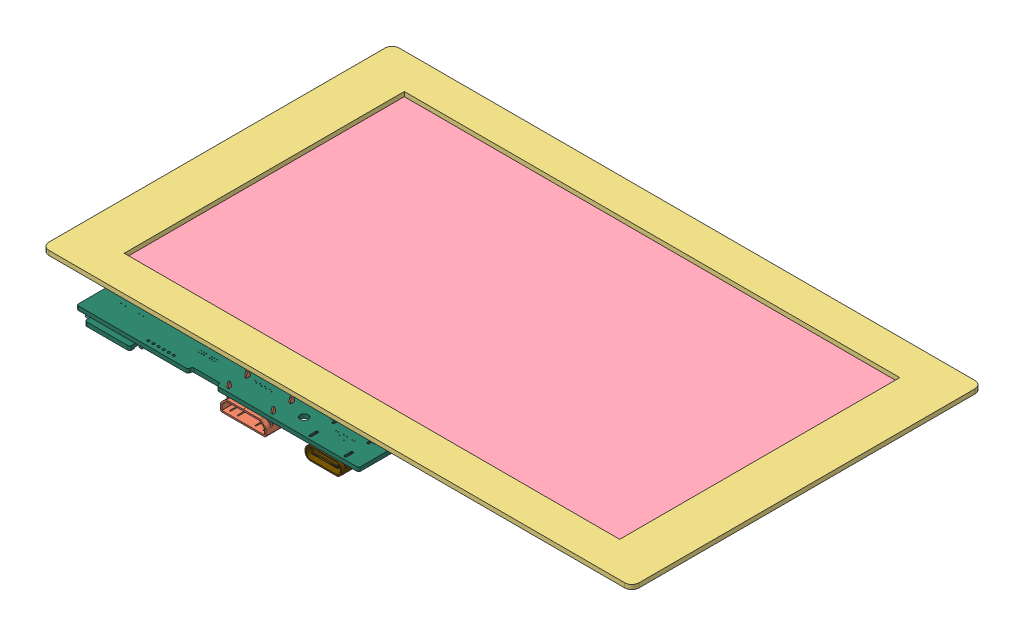
SolidWorks assembly Assembly Center Components, configuration Default. Lengths in mm.
Overall size (146.77 13.35 93.89).
640 component instances, 141 part files, 3 mates.
Components (placement in the parent):
- Mini HDMI 685119136923-1: Mini HDMI 685119136923 [Default] at (-19.19 -7.55 40.38) x (0 0 1) z (0 -1 0) size (7.9 11.25 5.45)
  - Mini HDMI 685119136923(1)-1: Mini HDMI 685119136923(1) [Default] at origin size (7.9 11.25 5.45)
    - Housing-1: Housing [Default] at origin size (5.5 11.25 2.9)
    - Shielding-1: Shielding [Default] at (2.875 0 0.82) x (0 1 0) z (0 0 1) size (11.21 7.6 5.45)
    - Housing2-1: Housing2 [Default] at (-0.075 0 -0.65) x (0 -1 0) z (0 0 1) size (8.25 0.75 1.6)
    - Pin1-1: Pin1 [Default] at (2.1 -3.6 0.3) size (5.9 0.15 1.8)
    - Pin1-2: Pin1 [Default] at (2.1 -2.8 0.3) size (5.9 0.15 1.8)
    - Pin1-3: Pin1 [Default] at (2.1 -2.4 0.3) size (5.9 0.15 1.8)
    - Pin1-4: Pin1 [Default] at (2.1 -2 0.3) size (5.9 0.15 1.8)
    - Pin1-5: Pin1 [Default] at (2.1 -1.6 0.3) size (5.9 0.15 1.8)
    - Pin1-6: Pin1 [Default] at (2.1 -1.2 0.3) size (5.9 0.15 1.8)
    - Pin1-7: Pin1 [Default] at (2.1 -0.8 0.3) size (5.9 0.15 1.8)
    - Pin1-8: Pin1 [Default] at (2.1 -0.4 0.3) size (5.9 0.15 1.8)
    - Pin1-9: Pin1 [Default] at (2.1 0 0.3) size (5.9 0.15 1.8)
    - Pin1-10: Pin1 [Default] at (2.1 0.4 0.3) size (5.9 0.15 1.8)
    - Pin1-11: Pin1 [Default] at (2.1 0.8 0.3) size (5.9 0.15 1.8)
    - Pin1-12: Pin1 [Default] at (2.1 1.2 0.3) size (5.9 0.15 1.8)
    - Pin1-13: Pin1 [Default] at (2.1 1.6 0.3) size (5.9 0.15 1.8)
    - Pin1-14: Pin1 [Default] at (2.1 2 0.3) size (5.9 0.15 1.8)
    - Pin1-15: Pin1 [Default] at (2.1 2.4 0.3) size (5.9 0.15 1.8)
    - Pin1-16: Pin1 [Default] at (2.1 2.8 0.3) size (5.9 0.15 1.8)
    - Pin1-17: Pin1 [Default] at (2.1 3.2 0.3) size (5.9 0.15 1.8)
    - Pin1-18: Pin1 [Default] at (2.1 3.6 0.3) size (5.9 0.15 1.8)
    - Pin2-1: Pin2 [Default] at (1.7983 -3.2 0.3) size (5.3 0.15 1.8)
- AX210 PCIe Card-1: AX210 PCIe Card [Default] at (0 25.3 -0.4) size (22 0.1 30)
  - Component473-1: Component473 [Default] at origin size (0.15 0.02 2.3)
  - Component424-1: Component424 [Default] at origin size (0.15 0.02 2.3)
  - Component429-1: Component429 [Default] at origin size (0.15 0.02 2.3)
  - Component423-1: Component423 [Default] at origin size (0.15 0.02 2.3)
  - Component430-1: Component430 [Default] at origin size (0.15 0.02 2.3)
  - Component431-1: Component431 [Default] at origin size (0.15 0.02 2.3)
  - Component426-1: Component426 [Default] at origin size (0.15 0.02 2.3)
  - Component422-1: Component422 [Default] at origin size (0.15 0.02 2.3)
  - Component425-1: Component425 [Default] at origin size (0.15 0.02 2.3)
  - Component428-1: Component428 [Default] at origin size (0.15 0.02 2.3)
  - Component446-1: Component446 [Default] at origin size (0.15 0.02 2.3)
  - Component448-1: Component448 [Default] at origin size (0.15 0.02 2.3)
  - Component449-1: Component449 [Default] at origin size (0.15 0.02 2.3)
  - Component443-1: Component443 [Default] at origin size (0.15 0.02 2.3)
  - Component442-1: Component442 [Default] at origin size (0.15 0.02 2.3)
  - Component447-1: Component447 [Default] at origin size (0.15 0.02 2.3)
  - Component451-1: Component451 [Default] at origin size (0.15 0.02 2.3)
  - Component450-1: Component450 [Default] at origin size (0.15 0.02 2.3)
  - Component445-1: Component445 [Default] at origin size (0.15 0.02 2.3)
  - Component472-1: Component472 [Default] at origin size (0.15 0.02 2.3)
  - Component408-1: Component408 [Default] at origin size (0.15 0.02 2.3)
  - Component409-1: Component409 [Default] at origin size (0.15 0.02 2.3)
  - Component410-1: Component410 [Default] at origin size (0.15 0.02 2.3)
  - Component405-1: Component405 [Default] at origin size (0.15 0.02 2.3)
  - Component411-1: Component411 [Default] at origin size (0.15 0.02 2.3)
  - Component403-1: Component403 [Default] at origin size (0.15 0.02 2.3)
  - Component406-1: Component406 [Default] at origin size (0.15 0.02 2.3)
  - Component404-1: Component404 [Default] at origin size (0.15 0.02 2.3)
  - Component407-1: Component407 [Default] at origin size (0.15 0.02 2.3)
  - Component400-1: Component400 [Default] at origin size (0.15 0.02 2.3)
  - Component401-1: Component401 [Default] at origin size (0.15 0.02 2.3)
  - Component433-1: Component433 [Default] at origin size (0.15 0.02 2.3)
  - Component437-1: Component437 [Default] at origin size (0.15 0.02 2.3)
  - Component438-1: Component438 [Default] at origin size (0.15 0.02 2.3)
  - Component436-1: Component436 [Default] at origin size (0.15 0.02 2.3)
  - Component434-1: Component434 [Default] at origin size (0.15 0.02 2.3)
  - Component439-1: Component439 [Default] at origin size (0.15 0.02 2.3)
  - Component440-1: Component440 [Default] at origin size (0.15 0.02 2.3)
  - Component435-1: Component435 [Default] at origin size (0.15 0.02 2.3)
  - Component458-1: Component458 [Default] at origin size (0.15 0.02 2.3)
  - Component460-1: Component460 [Default] at origin size (0.15 0.02 2.3)
  - Component456-1: Component456 [Default] at origin size (0.15 0.02 2.3)
  - Component457-1: Component457 [Default] at origin size (0.15 0.02 2.3)
  - Component461-1: Component461 [Default] at origin size (0.15 0.02 2.3)
  - Component452-1: Component452 [Default] at origin size (0.15 0.02 2.3)
  - Component453-1: Component453 [Default] at origin size (0.15 0.02 2.3)
  - Component455-1: Component455 [Default] at origin size (0.15 0.02 2.3)
  - Component465-1: Component465 [Default] at origin size (0.15 0.02 2.3)
  - Component468-1: Component468 [Default] at origin size (0.15 0.02 2.3)
  - Component467-1: Component467 [Default] at origin size (0.15 0.02 2.3)
  - Component464-1: Component464 [Default] at origin size (0.15 0.02 2.3)
  - Component469-1: Component469 [Default] at origin size (0.15 0.02 2.3)
  - Component470-1: Component470 [Default] at origin size (0.15 0.02 2.3)
  - Component471-1: Component471 [Default] at origin size (0.15 0.02 2.3)
  - Component462-1: Component462 [Default] at origin size (0.15 0.02 2.3)
  - Component463-1: Component463 [Default] at origin size (0.15 0.02 2.3)
  - Component466-1: Component466 [Default] at origin size (0.15 0.02 2.3)
  - Component413-1: Component413 [Default] at origin size (0.15 0.02 2.3)
  - Component417-1: Component417 [Default] at origin size (0.15 0.02 2.3)
  - Component414-1: Component414 [Default] at origin size (0.15 0.02 2.3)
  - Component415-1: Component415 [Default] at origin size (0.15 0.02 2.3)
  - Component421-1: Component421 [Default] at origin size (0.15 0.02 2.3)
  - Component418-1: Component418 [Default] at origin size (0.15 0.02 2.3)
  - Component419-1: Component419 [Default] at origin size (0.15 0.02 2.3)
  - Component420-1: Component420 [Default] at origin size (0.15 0.02 2.3)
  - Component412-1: Component412 [Default] at origin size (0.15 0.02 2.3)
  - AX210 PCIe Card-0-1: AX210 PCIe Card-0 [Default] at origin size (0.15 0.02 2.3)
  - AX210 PCIe Card-1-1: AX210 PCIe Card-1 [Default] at origin size (5.53 0.08 2.73)
  - AX210 PCIe Card-2-1: AX210 PCIe Card-2 [Default] at origin size (22 0.08 30)
- 5.5_ Touch Display MIPI-1: 5.5_ Touch Display MIPI [Default] at origin size (145.01 5.25 86.09)
  - CTP-1: CTP [Default] at origin size (145.01 1.1 86.09)
  - 5.5_ Touch Display MIPI-3-1: 5.5_ Touch Display MIPI-3 [Default] at origin size (133.31 3.65 74.36)
  - 5.5_ Touch Display MIPI-4-1: 5.5_ Touch Display MIPI-4 [Default] at origin size (45 0.5 15.5)
  - 5.5_ Touch Display MIPI-5-1: 5.5_ Touch Display MIPI-5 [Default] at origin size (53.5 0.5 4.5)
- RNQ0040A v1-1: RNQ0040A v1 [Default] at (1.8323 -6.1 22.7032) x (1 0 0) z (0 -1 0) size (6 4 0.8)
  - BODY-QFN-1: BODY-QFN [Default] at (0 0 0.025) x (1 0 0) z (0 -1 0) size (6 0.78 4)
  - FRAME-RNQ0040A-1: FRAME-RNQ0040A [Default] x (1 0 0) z (0 -1 0) size (6 0.2 4)
- Radxa CM3-1: Radxa CM3 [Default] at (-34.1679 -8.7691 -17.6603) x (0 0 -1) z (0 -1 0) size (40.05 55.02 3.7)
  - Board_Geoms-1: Board_Geoms [Default] at origin size (40.05 55.02 1.2)
    - Board_outline-1: Board_outline [Default] at origin size (40.05 55.02 1.2)
  - EMP_Models-1: EMP_Models [Default] at origin size (39.5 54.73 3.7)
    - ANT2-1: ANT2 [Default] at (-11.75 25.8 0) size (4.01 3.43 1.3)
    - C1-1: C1 [Default] at (-3.8475 -1.7481 -1.2) x (-0.707107 -0.707107 0) z (0 0 -1) size (1.7 0.9 0.5)
    - C10-1: C10 [Default] at (3.3025 0.0519 -1.2) x (0.707107 0.707107 0) z (0 0 -1) size (1.1 0.6 0.35)
    - C10-2: C10 [Default] at (10.95 15.45 -1.2) x (0 1 0) z (0 0 -1) size (1.1 0.6 0.35)
    - C10-3: C10 [Default] at (3.8025 -0.3981 -1.2) x (-0.707107 -0.707107 0) z (0 0 -1) size (1.1 0.6 0.35)
    - C10-4: C10 [Default] at (-3.9975 -0.8481 -1.2) x (0.707107 0.707107 0) z (0 0 -1) size (1.1 0.6 0.35)
    - C1-2: C1 [Default] at (-14.1389 2.0823 0) x (0 1 0) z (0 0 1) size (1.7 0.9 0.5)
    - C10-5: C10 [Default] at (-4.6975 -21.9981 -1.2) x (0.707107 0.707107 0) z (0 0 -1) size (1.1 0.6 0.35)
    - C105-1: C105 [Default] at (13.9593 20.2111 -1.2) x (1 0 0) z (0 0 -1) size (2.5 1.3 0.6)
    - C105-2: C105 [Default] at (0.7006 -26.6671 0) size (2.5 1.3 0.6)
    - C105-3: C105 [Default] at (3.9693 -10.6117 -1.2) x (0 1 0) z (0 0 -1) size (2.5 1.3 0.6)
    - C10-6: C10 [Default] at (-3.0975 -8.9981 -1.2) x (0 1 0) z (0 0 -1) size (1.1 0.6 0.35)
    - C10-7: C10 [Default] at (-2.3475 -3.2981 -1.2) x (-0.707107 -0.707107 0) z (0 0 -1) size (1.1 0.6 0.35)
    - C1-3: C1 [Default] at (3.0025 0.7019 -1.2) x (0.707107 0.707107 0) z (0 0 -1) size (1.7 0.9 0.5)
    - C10-8: C10 [Default] at (-1.4475 -4.5481 -1.2) x (-0.707107 -0.707107 0) z (0 0 -1) size (1.1 0.6 0.35)
    - C10-9: C10 [Default] at (0.4525 -5.1481 -1.2) x (-0.707107 -0.707107 0) z (0 0 -1) size (1.1 0.6 0.35)
    - C10-10: C10 [Default] at (1.1525 -20.3481 -1.2) x (0 1 0) z (0 0 -1) size (1.1 0.6 0.35)
    - C10-11: C10 [Default] at (-2.0975 -16.8481 -1.2) x (0 1 0) z (0 0 -1) size (1.1 0.6 0.35)
    - C10-12: C10 [Default] at (-8.6975 -22.5481 -1.2) x (0.707107 -0.707107 0) z (0 0 -1) size (1.1 0.6 0.35)
    - C10-13: C10 [Default] at (-1.7475 -19.9981 -1.2) x (0.707107 -0.707107 0) z (0 0 -1) size (1.1 0.6 0.35)
    - C10-14: C10 [Default] at (2.6525 -20.0481 -1.2) x (1 0 0) z (0 0 -1) size (1.1 0.6 0.35)
    - C10-15: C10 [Default] at (6.7025 -17.4981 -1.2) x (0 1 0) z (0 0 -1) size (1.1 0.6 0.35)
    - C10-16: C10 [Default] at (-3.1475 -12.2481 0) x (0 -1 0) z (0 0 1) size (1.1 0.6 0.35)
    - C10-17: C10 [Default] at (-2.4475 -25.0481 -1.2) x (0.707107 -0.707107 0) z (0 0 -1) size (1.1 0.6 0.35)
    - C105-4: C105 [Default] at (0.9025 1.6519 -1.2) x (-0.707107 0.707107 0) z (0 0 -1) size (2.5 1.3 0.6)
    - C10-18: C10 [Default] at (-3.9475 -20.1981 -1.2) x (-0.707107 0.707107 0) z (0 0 -1) size (1.1 0.6 0.35)
    - C10-19: C10 [Default] at (6.3025 -22.0481 -1.2) x (0 -1 0) z (0 0 -1) size (1.1 0.6 0.35)
    - C10-20: C10 [Default] at (2.2025 -13.4481 -1.2) x (0 1 0) z (0 0 -1) size (1.1 0.6 0.35)
    - C10-21: C10 [Default] at (-3.4975 -13.6981 -1.2) x (0 1 0) z (0 0 -1) size (1.1 0.6 0.35)
    - C10-22: C10 [Default] at (-0.8475 -23.4481 -1.2) x (0.707107 -0.707107 0) z (0 0 -1) size (1.1 0.6 0.35)
    - C105-5: C105 [Default] at (3.682 -21.4585 -1.2) x (-1 0 0) z (0 0 -1) size (2.5 1.3 0.6)
    - C105-6: C105 [Default] at (-7.2334 -17.3788 -1.2) x (0 1 0) z (0 0 -1) size (2.5 1.3 0.6)
    - C105-7: C105 [Default] at (-10.5087 -5.7093 -1.2) x (-0.707107 -0.707107 0) z (0 0 -1) size (2.5 1.3 0.6)
    - C10-23: C10 [Default] at (8.2025 -12.0481 -1.2) x (0 1 0) z (0 0 -1) size (1.1 0.6 0.35)
    - C10-24: C10 [Default] at (-0.6475 -3.2981 -1.2) x (-0.707107 -0.707107 0) z (0 0 -1) size (1.1 0.6 0.35)
    - C105-8: C105 [Default] at (9 7.85 -1.2) x (1 0 0) z (0 0 -1) size (2.5 1.3 0.6)
    - C10-25: C10 [Default] at (1.1025 -3.3981 -1.2) x (0.707107 -0.707107 0) z (0 0 -1) size (1.1 0.6 0.35)
    - C10-26: C10 [Default] at (1.5525 -2.8981 -1.2) x (0.707107 -0.707107 0) z (0 0 -1) size (1.1 0.6 0.35)
    - C10-27: C10 [Default] at (5.7025 -24.2481 -1.2) x (-1 0 0) z (0 0 -1) size (1.1 0.6 0.35)
    - C10-28: C10 [Default] at (-9.6087 -6.0593 -1.2) x (-0.707107 -0.707107 0) z (0 0 -1) size (1.1 0.6 0.35)
    - C10-29: C10 [Default] at (5.3525 -16.2481 -1.2) x (0.707107 0.707107 0) z (0 0 -1) size (1.1 0.6 0.35)
    - C10-30: C10 [Default] at (4.1025 -19.8481 -1.2) x (0 -1 0) z (0 0 -1) size (1.1 0.6 0.35)
    - C10-31: C10 [Default] at (5.2525 -18.4981 -1.2) x (-1 0 0) z (0 0 -1) size (1.1 0.6 0.35)
    - C10-32: C10 [Default] at (-7.9475 -21.8981 -1.2) x (-0.707107 0.707107 0) z (0 0 -1) size (1.1 0.6 0.35)
    - C10-33: C10 [Default] at (-7.8975 -11.9481 -1.2) x (-0.707107 -0.707107 0) z (0 0 -1) size (1.1 0.6 0.35)
    - C10-34: C10 [Default] at (2.8025 -23.5481 -1.2) x (0 -1 0) z (0 0 -1) size (1.1 0.6 0.35)
    - C10-35: C10 [Default] at (-2.6475 1.2519 -1.2) x (0.707107 -0.707107 0) z (0 0 -1) size (1.1 0.6 0.35)
    - C10-36: C10 [Default] at (4.0025 -24.9981 -1.2) x (-1 0 0) z (0 0 -1) size (1.1 0.6 0.35)
    - C10-37: C10 [Default] at (-12.1475 -16.9481 -1.2) x (0 -1 0) z (0 0 -1) size (1.1 0.6 0.35)
    - C10-38: C10 [Default] at (4.2525 -14.4981 -1.2) x (1 0 0) z (0 0 -1) size (1.1 0.6 0.35)
    - C10-39: C10 [Default] at (8.2025 -19.6981 -1.2) x (0 1 0) z (0 0 -1) size (1.1 0.6 0.35)
    - C10-40: C10 [Default] at (3.8025 -17.7981 -1.2) x (1 0 0) z (0 0 -1) size (1.1 0.6 0.35)
    - C10-41: C10 [Default] at (-7.0975 -20.8481 -1.2) x (-0.707107 0.707107 0) z (0 0 -1) size (1.1 0.6 0.35)
    - C10-42: C10 [Default] at (-6.5975 -15.0481 -1.2) x (-0.707107 0.707107 0) z (0 0 -1) size (1.1 0.6 0.35)
    - C105-9: C105 [Default] at (11.9 -25.25 -1.2) x (1 0 0) z (0 0 -1) size (2.5 1.3 0.6)
    - C10-43: C10 [Default] at (-2.9975 -22.1481 -1.2) x (1 0 0) z (0 0 -1) size (1.1 0.6 0.35)
    - C10-44: C10 [Default] at (-17.9 -20.3 -1.2) x (1 0 0) z (0 0 -1) size (1.1 0.6 0.35)
    - C105-10: C105 [Default] at (-1.4475 2.3019 -1.2) x (0.707107 0.707107 0) z (0 0 -1) size (2.5 1.3 0.6)
    - C105-11: C105 [Default] at (1.5025 -25.9481 -1.2) x (1 0 0) z (0 0 -1) size (2.5 1.3 0.6)
    - C10-45: C10 [Default] at (3.4525 -15.6981 -1.2) x (1 0 0) z (0 0 -1) size (1.1 0.6 0.35)
    - C10-46: C10 [Default] at (-4.7975 -24.2981 -1.2) x (-0.707107 -0.707107 0) z (0 0 -1) size (1.1 0.6 0.35)
    - C10-47: C10 [Default] at (12.7525 -26.8981 -1.2) x (1 0 0) z (0 0 -1) size (1.1 0.6 0.35)
    - C105-12: C105 [Default] at (8.9525 -25.6481 -1.2) x (0 1 0) z (0 0 -1) size (2.5 1.3 0.6)
    - C1-4: C1 [Default] at (-15.75 -20.3 -1.2) x (-1 0 0) z (0 0 -1) size (1.7 0.9 0.5)
    - C105-13: C105 [Default] at (-4.3502 -26.0128 -1.2) x (-0.707107 -0.707107 0) z (0 0 -1) size (2.5 1.3 0.6)
    - C10-48: C10 [Default] at (2.5525 -18.8981 -1.2) x (1 0 0) z (0 0 -1) size (1.1 0.6 0.35)
    - C10-49: C10 [Default] at (1.7025 -23.5481 -1.2) x (0 1 0) z (0 0 -1) size (1.1 0.6 0.35)
    - C10-50: C10 [Default] at (-4.6475 -15.4981 -1.2) x (0 1 0) z (0 0 -1) size (1.1 0.6 0.35)
    - C105-14: C105 [Default] at (-2.8975 3.4519 -1.2) x (-0.707107 0.707107 0) z (0 0 -1) size (2.5 1.3 0.6)
    - C10-51: C10 [Default] at (-15.6 -16.6 -1.2) x (-1 0 0) z (0 0 -1) size (1.1 0.6 0.35)
    - C10-52: C10 [Default] at (11.5525 -22.4481 0) x (-1 0 0) z (0 0 1) size (1.1 0.6 0.35)
    - C10-53: C10 [Default] at (-17.25 -16.6 -1.2) x (1 0 0) z (0 0 -1) size (1.1 0.6 0.35)
    - C10-54: C10 [Default] at (-9.6071 3.2927 -1.2) x (0 1 0) z (0 0 -1) size (1.1 0.6 0.35)
    - C10-55: C10 [Default] at (-10.9034 6.1115 -1.2) x (0 1 0) z (0 0 -1) size (1.1 0.6 0.35)
    - C1-5: C1 [Default] at (-14.1734 12.7084 -1.2) x (0 -1 0) z (0 0 -1) size (1.7 0.9 0.5)
    - C1-6: C1 [Default] at (-5.1488 16.5367 0) x (0 1 0) z (0 0 1) size (1.7 0.9 0.5)
    - C10-56: C10 [Default] at (3.6525 -2.8981 -1.2) x (0.707107 0.707107 0) z (0 0 -1) size (1.1 0.6 0.35)
    - C1-7: C1 [Default] at (-7.1 20.8 0) size (1.7 0.9 0.5)
    - C10-57: C10 [Default] at (-8.4 20.75 0) x (-1 0 0) z (0 0 1) size (1.1 0.6 0.35)
    - C1-8: C1 [Default] at (6.8025 -3.5481 -1.2) x (-1 0 0) z (0 0 -1) size (1.7 0.9 0.5)
    - C10-58: C10 [Default] at (-5.1475 -1.2981 -1.2) x (-0.707107 0.707107 0) z (0 0 -1) size (1.1 0.6 0.35)
    - C10-59: C10 [Default] at (-14.45 -15.95 -1.2) x (1 0 0) z (0 0 -1) size (1.1 0.6 0.35)
    - C10-60: C10 [Default] at (13.1787 3.2726 -1.2) x (1 0 0) z (0 0 -1) size (1.1 0.6 0.35)
    - C105-15: C105 [Default] at (-14.4642 14.7415 -1.2) x (0 -1 0) z (0 0 -1) size (2.5 1.3 0.6)
    - C10-61: C10 [Default] at (-15.3485 19.4403 -1.2) x (0 1 0) z (0 0 -1) size (1.1 0.6 0.35)
    - C10-62: C10 [Default] at (-11.4987 22.5227 0) x (0 1 0) z (0 0 1) size (1.1 0.6 0.35)
    - C105-16: C105 [Default] at (-14.4738 19.5134 -1.2) x (0 1 0) z (0 0 -1) size (2.5 1.3 0.6)
    - C10-63: C10 [Default] at (-17.1616 18.5714 -1.2) x (1 0 0) z (0 0 -1) size (1.1 0.6 0.35)
    - C10-64: C10 [Default] at (-18.3116 18.5714 -1.2) x (-1 0 0) z (0 0 -1) size (1.1 0.6 0.35)
    - C10-65: C10 [Default] at (-19.0475 6.1019 0) x (-1 0 0) z (0 0 1) size (1.1 0.6 0.35)
    - C1-9: C1 [Default] at (5.4525 -4.1481 -1.2) x (0 1 0) z (0 0 -1) size (1.7 0.9 0.5)
    - C10-66: C10 [Default] at (-19.0475 6.7019 0) x (-1 0 0) z (0 0 1) size (1.1 0.6 0.35)
    - C10-67: C10 [Default] at (-17.8088 2.3575 0) x (-1 0 0) z (0 0 1) size (1.1 0.6 0.35)
    - C1-10: C1 [Default] at (-17.1397 6.6977 0) size (1.7 0.9 0.5)
    - C10-68: C10 [Default] at (-16.0385 6.7928 0) x (0 -1 0) z (0 0 1) size (1.1 0.6 0.35)
    - C10-69: C10 [Default] at (18.6 -11.05 0) x (0 1 0) z (0 0 1) size (1.1 0.6 0.35)
    - C10-70: C10 [Default] at (18.75 -15.6 0) size (1.1 0.6 0.35)
    - C10-71: C10 [Default] at (18.2 -16.1 -1.2) x (-1 0 0) z (0 0 -1) size (1.1 0.6 0.35)
    - C10-72: C10 [Default] at (18.75 -16.75 0) size (1.1 0.6 0.35)
    - C10-73: C10 [Default] at (18.75 -16.1 0) size (1.1 0.6 0.35)
    - C10-74: C10 [Default] at (-8.2975 -17.0981 -1.2) x (0 1 0) z (0 0 -1) size (1.1 0.6 0.35)
    - C10-75: C10 [Default] at (18.7502 -17.3853 0) size (1.1 0.6 0.35)
    - C1-11: C1 [Default] at (13.5025 -6.8481 0) size (1.7 0.9 0.5)
    - C1-12: C1 [Default] at (14.4525 -9.6481 0) size (1.7 0.9 0.5)
    - C10-76: C10 [Default] at (15.8525 -20.1981 0) x (0 -1 0) z (0 0 1) size (1.1 0.6 0.35)
    - C10-77: C10 [Default] at (15.8525 -20.1981 -1.2) x (0 -1 0) z (0 0 -1) size (1.1 0.6 0.35)
    - C1-13: C1 [Default] at (14.75 -11.85 -1.2) x (1 0 0) z (0 0 -1) size (1.7 0.9 0.5)
    - C1-14: C1 [Default] at (12.9525 -12.7981 -1.2) x (1 0 0) z (0 0 -1) size (1.7 0.9 0.5)
    - C10-78: C10 [Default] at (17.5 -13.4 -1.2) x (-1 0 0) z (0 0 -1) size (1.1 0.6 0.35)
    - C10-79: C10 [Default] at (12.8025 -13.5981 -1.2) x (1 0 0) z (0 0 -1) size (1.1 0.6 0.35)
    - C1-15: C1 [Default] at (18.8525 -20.0981 -1.2) x (-1 0 0) z (0 0 -1) size (1.7 0.9 0.5)
    - C1-16: C1 [Default] at (-3.0475 -2.3481 -1.2) x (-0.707107 -0.707107 0) z (0 0 -1) size (1.7 0.9 0.5)
    - C10-80: C10 [Default] at (0.4525 -18.5981 -1.2) x (-0.707107 -0.707107 0) z (0 0 -1) size (1.1 0.6 0.35)
    - C10-81: C10 [Default] at (18.9025 -20.8981 -1.2) x (-1 0 0) z (0 0 -1) size (1.1 0.6 0.35)
    - C10-82: C10 [Default] at (14.3025 -13.4481 -1.2) x (0 -1 0) z (0 0 -1) size (1.1 0.6 0.35)
    - C10-83: C10 [Default] at (12.8025 -14.2981 -1.2) x (1 0 0) z (0 0 -1) size (1.1 0.6 0.35)
    - C1-17: C1 [Default] at (17.0525 -20.0981 -1.2) x (1 0 0) z (0 0 -1) size (1.7 0.9 0.5)
    - C10-84: C10 [Default] at (16.5025 -20.1981 0) x (0 -1 0) z (0 0 1) size (1.1 0.6 0.35)
    - C10-85: C10 [Default] at (12.9025 -16.2481 -1.2) x (1 0 0) z (0 0 -1) size (1.1 0.6 0.35)
    - C10-86: C10 [Default] at (14.9912 -13.4244 -1.2) x (0 -1 0) z (0 0 -1) size (1.1 0.6 0.35)
    - C10-87: C10 [Default] at (17.5 -14.7 -1.2) x (-1 0 0) z (0 0 -1) size (1.1 0.6 0.35)
    - C10-88: C10 [Default] at (13.1025 -17.9981 -1.2) x (0 1 0) z (0 0 -1) size (1.1 0.6 0.35)
    - C10-89: C10 [Default] at (14.5525 -20.1981 0) x (0 -1 0) z (0 0 1) size (1.1 0.6 0.35)
    - C10-90: C10 [Default] at (0.0025 -12.9481 -1.2) x (0 1 0) z (0 0 -1) size (1.1 0.6 0.35)
    - C1-18: C1 [Default] at (-0.1475 -4.5981 -1.2) x (-0.707107 -0.707107 0) z (0 0 -1) size (1.7 0.9 0.5)
    - C10-91: C10 [Default] at (8.65 16.75 -1.2) x (-1 0 0) z (0 0 -1) size (1.1 0.6 0.35)
    - C10-92: C10 [Default] at (8.65 16.25 -1.2) x (-1 0 0) z (0 0 -1) size (1.1 0.6 0.35)
    - C105-17: C105 [Default] at (-17.9775 -6.6601 0) x (-0.707107 0.707107 0) z (0 0 1) size (2.5 1.3 0.6)
    - C105-18: C105 [Default] at (5.85 15.5 -1.2) x (0 1 0) z (0 0 -1) size (2.5 1.3 0.6)
    - C10-93: C10 [Default] at (3.7 14.75 -1.2) x (0 1 0) z (0 0 -1) size (1.1 0.6 0.35)
    - C10-94: C10 [Default] at (10.45 15.45 -1.2) x (0 1 0) z (0 0 -1) size (1.1 0.6 0.35)
    - C1-19: C1 [Default] at (10.6615 18.7103 -1.2) x (1 0 0) z (0 0 -1) size (1.7 0.9 0.5)
    - C10-95: C10 [Default] at (11.05 13.4 0) x (0 1 0) z (0 0 1) size (1.1 0.6 0.35)
    - C105-19: C105 [Default] at (9.65 12.3 -1.2) x (-1 0 0) z (0 0 -1) size (2.5 1.3 0.6)
    - C105-20: C105 [Default] at (0.1 0.75 -1.2) x (-0.707107 0.707107 0) z (0 0 -1) size (2.5 1.3 0.6)
    - C105-21: C105 [Default] at (-2.75 16.8 0) x (0 -1 0) z (0 0 1) size (2.5 1.3 0.6)
    - C105-22: C105 [Default] at (-4.1 16.8 0) x (0 -1 0) z (0 0 1) size (2.5 1.3 0.6)
    - C10-96: C10 [Default] at (8.5825 19.1459 -1.2) x (-1 0 0) z (0 0 -1) size (1.1 0.6 0.35)
    - C10-97: C10 [Default] at (8.55 19.8 -1.2) x (-1 0 0) z (0 0 -1) size (1.1 0.6 0.35)
    - C10-98: C10 [Default] at (8.6013 20.3134 -1.2) x (-1 0 0) z (0 0 -1) size (1.1 0.6 0.35)
    - C10-99: C10 [Default] at (3.2 14.75 -1.2) x (0 1 0) z (0 0 -1) size (1.1 0.6 0.35)
    - C105-23: C105 [Default] at (11.85 16.95 -1.2) x (1 0 0) z (0 0 -1) size (2.5 1.3 0.6)
    - C10-100: C10 [Default] at (3.75 13.1 0) x (0 -1 0) z (0 0 1) size (1.1 0.6 0.35)
    - C10-101: C10 [Default] at (3.95 11.35 0) x (-1 0 0) z (0 0 1) size (1.1 0.6 0.35)
    - C105-24: C105 [Default] at (9 9.05 -1.2) x (1 0 0) z (0 0 -1) size (2.5 1.3 0.6)
    - C105-25: C105 [Default] at (15.2 18.25 -1.2) x (0 -1 0) z (0 0 -1) size (2.5 1.3 0.6)
    - C10-102: C10 [Default] at (5.8 13.2 -1.2) x (0 -1 0) z (0 0 -1) size (1.1 0.6 0.35)
    - C10-103: C10 [Default] at (4.25 13.1 0) x (0 -1 0) z (0 0 1) size (1.1 0.6 0.35)
    - C105-26: C105 [Default] at (7.05 10.45 -1.2) x (0 1 0) z (0 0 -1) size (2.5 1.3 0.6)
    - C105-27: C105 [Default] at (-1.2753 -24.5477 -1.2) x (-0.707107 0.707107 0) z (0 0 -1) size (2.5 1.3 0.6)
    - C10-104: C10 [Default] at (2.9963 23.8177 0) x (0 1 0) z (0 0 1) size (1.1 0.6 0.35)
    - C105-28: C105 [Default] at (11.0433 21.7332 0) size (2.5 1.3 0.6)
    - C105-29: C105 [Default] at (2.5 20.95 -1.2) x (1 0 0) z (0 0 -1) size (2.5 1.3 0.6)
    - C10-105: C10 [Default] at (7.4413 23.0557 0) x (-1 0 0) z (0 0 1) size (1.1 0.6 0.35)
    - C10-106: C10 [Default] at (5.7 26.4 0) x (0 1 0) z (0 0 1) size (1.1 0.6 0.35)
    - C105-30: C105 [Default] at (2.5 19.75 -1.2) x (1 0 0) z (0 0 -1) size (2.5 1.3 0.6)
    - C105-31: C105 [Default] at (-4.1 20.65 0) x (0 -1 0) z (0 0 1) size (2.5 1.3 0.6)
    - C105-32: C105 [Default] at (-2.9 20.65 0) x (0 -1 0) z (0 0 1) size (2.5 1.3 0.6)
    - C10-107: C10 [Default] at (6.4683 25.0097 0) x (0 1 0) z (0 0 1) size (1.1 0.6 0.35)
    - C10-108: C10 [Default] at (9.4074 24.6986 0) x (0 1 0) z (0 0 1) size (1.1 0.6 0.35)
    - C10-109: C10 [Default] at (7.4413 23.9447 0) x (-1 0 0) z (0 0 1) size (1.1 0.6 0.35)
    - C10-110: C10 [Default] at (2.9963 24.9607 0) x (0 -1 0) z (0 0 1) size (1.1 0.6 0.35)
    - C105-33: C105 [Default] at (-5.35 24.95 0) size (2.5 1.3 0.6)
    - C10-111: C10 [Default] at (2.3613 23.8177 0) x (0 1 0) z (0 0 1) size (1.1 0.6 0.35)
    - C10-112: C10 [Default] at (1.1432 23.4631 0) size (1.1 0.6 0.35)
    - C10-113: C10 [Default] at (3.8853 24.9607 0) x (0 -1 0) z (0 0 1) size (1.1 0.6 0.35)
    - C10-114: C10 [Default] at (11.0479 19.812 -1.2) x (-1 0 0) z (0 0 -1) size (1.1 0.6 0.35)
    - C10-115: C10 [Default] at (0.0003 23.4631 0) x (-1 0 0) z (0 0 1) size (1.1 0.6 0.35)
    - C10-116: C10 [Default] at (4.5203 23.8177 0) x (0 -1 0) z (0 0 1) size (1.1 0.6 0.35)
    - C10-117: C10 [Default] at (1.6 16.7 -1.2) x (-1 0 0) z (0 0 -1) size (1.1 0.6 0.35)
    - C10-118: C10 [Default] at (5.2823 24.9607 0) x (0 -1 0) z (0 0 1) size (1.1 0.6 0.35)
    - C10-119: C10 [Default] at (3.8853 23.8177 0) x (0 1 0) z (0 0 1) size (1.1 0.6 0.35)
    - C10-120: C10 [Default] at (4.6473 24.9607 0) x (0 1 0) z (0 0 1) size (1.1 0.6 0.35)
    - C10-121: C10 [Default] at (-0.45 14.65 0) x (0 1 0) z (0 0 1) size (1.1 0.6 0.35)
    - C10-122: C10 [Default] at (-3.3387 23.8177 0) x (0 1 0) z (0 0 1) size (1.1 0.6 0.35)
    - C10-123: C10 [Default] at (-17.3087 -5.9093 0) x (-0.707107 0.707107 0) z (0 0 1) size (1.1 0.6 0.35)
    - C105-34: C105 [Default] at (7.9 17.65 -1.2) x (-1 0 0) z (0 0 -1) size (2.5 1.3 0.6)
    - C105-35: C105 [Default] at (17.8365 4.9199 0) x (0 -1 0) z (0 0 1) size (2.5 1.3 0.6)
    - C10-124: C10 [Default] at (17.9653 11.4831 0) size (1.1 0.6 0.35)
    - C105-36: C105 [Default] at (18.25 10.35 0) size (2.5 1.3 0.6)
    - C10-125: C10 [Default] at (-17.2504 -0.8345 0) x (-0.707107 -0.707107 0) z (0 0 1) size (1.1 0.6 0.35)
    - C105-37: C105 [Default] at (-12.05 -2.5 0) x (0.707107 -0.707107 0) z (0 0 1) size (2.5 1.3 0.6)
    - C105-38: C105 [Default] at (-14.7 -2.6 0) x (-0.707107 -0.707107 0) z (0 0 1) size (2.5 1.3 0.6)
    - C105-39: C105 [Default] at (-15.65 -1.6 0) x (-0.707107 -0.707107 0) z (0 0 1) size (2.5 1.3 0.6)
    - C10-126: C10 [Default] at (-17.6244 -3.2773 0) x (-0.707107 0.707107 0) z (0 0 1) size (1.1 0.6 0.35)
    - C10-127: C10 [Default] at (5 11.1 -1.2) x (0 -1 0) z (0 0 -1) size (1.1 0.6 0.35)
    - C10-128: C10 [Default] at (2.6 11.1 -1.2) x (0 -1 0) z (0 0 -1) size (1.1 0.6 0.35)
    - C10-129: C10 [Default] at (0.1 3.25 -1.2) x (-0.707107 -0.707107 0) z (0 0 -1) size (1.1 0.6 0.35)
    - C10-130: C10 [Default] at (3.4 11.1 -1.2) x (0 -1 0) z (0 0 -1) size (1.1 0.6 0.35)
    - C105-40: C105 [Default] at (-3.5 18.6 0) size (2.5 1.3 0.6)
    - C10-131: C10 [Default] at (14.25 -3.05 0) x (0 -1 0) z (0 0 1) size (1.1 0.6 0.35)
    - C105-41: C105 [Default] at (13.9025 -5.4981 0) size (2.5 1.3 0.6)
    - C10-132: C10 [Default] at (13.75 -4.65 0) size (1.1 0.6 0.35)
    - C105-42: C105 [Default] at (13.85 18.25 -1.2) x (0 -1 0) z (0 0 -1) size (2.5 1.3 0.6)
    - C10-133: C10 [Default] at (-5.2475 -23.8481 -1.2) x (-0.707107 -0.707107 0) z (0 0 -1) size (1.1 0.6 0.35)
    - C10-134: C10 [Default] at (-5.9475 -24.9981 -1.2) x (0.707107 -0.707107 0) z (0 0 -1) size (1.1 0.6 0.35)
    - C10-135: C10 [Default] at (5.3025 -8.0981 -1.2) x (1 0 0) z (0 0 -1) size (1.1 0.6 0.35)
    - C1-20: C1 [Default] at (0.5525 -2.4481 -1.2) x (0.707107 0.707107 0) z (0 0 -1) size (1.7 0.9 0.5)
    - C1-21: C1 [Default] at (-1.1651 -2.1207 -1.2) x (-0.707107 0.707107 0) z (0 0 -1) size (1.7 0.9 0.5)
    - C10-136: C10 [Default] at (0.1 14.65 0) x (0 1 0) z (0 0 1) size (1.1 0.6 0.35)
    - C105-43: C105 [Default] at (-3.5 0.5 -1.2) x (-0.707107 0.707107 0) z (0 0 -1) size (2.5 1.3 0.6)
    - C10-137: C10 [Default] at (-4.35 11.05 0) size (1.1 0.6 0.35)
    - C10-138: C10 [Default] at (-5.5038 11.0162 0) x (-1 0 0) z (0 0 1) size (1.1 0.6 0.35)
    - C10-139: C10 [Default] at (0.7025 5.2019 -1.2) x (0.707107 0.707107 0) z (0 0 -1) size (1.1 0.6 0.35)
    - C10-140: C10 [Default] at (-1.35 4.5 -1.2) x (-0.707107 -0.707107 0) z (0 0 -1) size (1.1 0.6 0.35)
    - C10-141: C10 [Default] at (-0.75 5.45 -1.2) x (0.707107 0.707107 0) z (0 0 -1) size (1.1 0.6 0.35)
    - C10-142: C10 [Default] at (-2.6 7.15 -1.2) x (-1 0 0) z (0 0 -1) size (1.1 0.6 0.35)
    - C10-143: C10 [Default] at (-1.7475 5.9519 -1.2) x (0.707107 -0.707107 0) z (0 0 -1) size (1.1 0.6 0.35)
    - C10-144: C10 [Default] at (8.25 14.15 -1.2) x (-1 0 0) z (0 0 -1) size (1.1 0.6 0.35)
    - C10-145: C10 [Default] at (-1.9975 4.1019 -1.2) x (0.707107 -0.707107 0) z (0 0 -1) size (1.1 0.6 0.35)
    - C10-146: C10 [Default] at (-1.1975 3.8019 -1.2) x (-0.707107 -0.707107 0) z (0 0 -1) size (1.1 0.6 0.35)
    - C105-44: C105 [Default] at (-1.5975 -0.3481 -1.2) x (0.707107 0.707107 0) z (0 0 -1) size (2.5 1.3 0.6)
    - C10-147: C10 [Default] at (1.95 -3.55 -1.2) x (-0.707107 -0.707107 0) z (0 0 -1) size (1.1 0.6 0.35)
    - C10-148: C10 [Default] at (2.3 -3.9 -1.2) x (-0.707107 -0.707107 0) z (0 0 -1) size (1.1 0.6 0.35)
    - C10-149: C10 [Default] at (-1.7 4.85 -1.2) x (-0.707107 -0.707107 0) z (0 0 -1) size (1.1 0.6 0.35)
    - C10-150: C10 [Default] at (-0.45 4.65 -1.2) x (0.707107 -0.707107 0) z (0 0 -1) size (1.1 0.6 0.35)
    - C10-151: C10 [Default] at (-14.45 -16.6 -1.2) x (1 0 0) z (0 0 -1) size (1.1 0.6 0.35)
    - C10-152: C10 [Default] at (-5.6475 1.4519 -1.2) x (-0.707107 -0.707107 0) z (0 0 -1) size (1.1 0.6 0.35)
    - C10-153: C10 [Default] at (-9.5877 22.6017 0) x (0 1 0) z (0 0 1) size (1.1 0.6 0.35)
    - C10-154: C10 [Default] at (-4.9838 2.7384 -1.2) x (-0.707107 -0.707107 0) z (0 0 -1) size (1.1 0.6 0.35)
    - C10-155: C10 [Default] at (-3.4533 2.4614 -1.2) x (0.707107 0.707107 0) z (0 0 -1) size (1.1 0.6 0.35)
    - C10-156: C10 [Default] at (-4.2975 3.6019 -1.2) x (-0.707107 0.707107 0) z (0 0 -1) size (1.1 0.6 0.35)
    - C10-157: C10 [Default] at (1.6525 -1.6481 -1.2) x (-0.707107 -0.707107 0) z (0 0 -1) size (1.1 0.6 0.35)
    - C10-158: C10 [Default] at (0.25 10.55 -1.2) x (0 1 0) z (0 0 -1) size (1.1 0.6 0.35)
    - C10-159: C10 [Default] at (-5.2818 15.3952 0) size (1.1 0.6 0.35)
    - C10-160: C10 [Default] at (3.4025 -2.2481 -1.2) x (0.707107 0.707107 0) z (0 0 -1) size (1.1 0.6 0.35)
    - C10-161: C10 [Default] at (2.8025 -1.6481 -1.2) x (-0.707107 0.707107 0) z (0 0 -1) size (1.1 0.6 0.35)
    - C10-162: C10 [Default] at (-6.7675 7.1519 0) x (-0.707107 0.707107 0) z (0 0 1) size (1.1 0.6 0.35)
    - C10-163: C10 [Default] at (-6.3865 7.5329 0) x (-0.707107 0.707107 0) z (0 0 1) size (1.1 0.6 0.35)
    - C10-164: C10 [Default] at (8.6535 15.7139 -1.2) x (-1 0 0) z (0 0 -1) size (1.1 0.6 0.35)
    - C10-165: C10 [Default] at (-5.4975 8.5489 0) x (-0.707107 0.707107 0) z (0 0 1) size (1.1 0.6 0.35)
    - C10-166: C10 [Default] at (-5.9125 8.0719 0) x (-0.707107 0.707107 0) z (0 0 1) size (1.1 0.6 0.35)
    - C10-167: C10 [Default] at (-2.6475 4.9519 -1.2) x (0.707107 -0.707107 0) z (0 0 -1) size (1.1 0.6 0.35)
    - C1-22: C1 [Default] at (0.2025 -1.3981 -1.2) x (-0.707107 -0.707107 0) z (0 0 -1) size (1.7 0.9 0.5)
    - C10-168: C10 [Default] at (2.0525 -2.0981 -1.2) x (0.707107 0.707107 0) z (0 0 -1) size (1.1 0.6 0.35)
    - C1-23: C1 [Default] at (8.3303 14.9277 -1.2) x (-1 0 0) z (0 0 -1) size (1.7 0.9 0.5)
    - C1-24: C1 [Default] at (0.9 11.1 -1.2) x (0 1 0) z (0 0 -1) size (1.7 0.9 0.5)
    - C10-169: C10 [Default] at (-12.4547 0.1177 0) x (0.707107 -0.707107 0) z (0 0 1) size (1.1 0.6 0.35)
    - C10-170: C10 [Default] at (-12.9047 -0.3323 0) x (0.707107 -0.707107 0) z (0 0 1) size (1.1 0.6 0.35)
    - C10-171: C10 [Default] at (-6.4948 1.7665 -1.2) x (0.707107 -0.707107 0) z (0 0 -1) size (1.1 0.6 0.35)
    - C10-172: C10 [Default] at (-9.7716 0.8527 -1.2) x (-1 0 0) z (0 0 -1) size (1.1 0.6 0.35)
    - C10-173: C10 [Default] at (-7.95 1 -1.2) x (-0.707107 0.707107 0) z (0 0 -1) size (1.1 0.6 0.35)
    - C10-174: C10 [Default] at (-9.7407 -1.0384 -1.2) x (-1 0 0) z (0 0 -1) size (1.1 0.6 0.35)
    - C10-175: C10 [Default] at (-5.8561 -0.2604 -1.2) x (-0.707107 -0.707107 0) z (0 0 -1) size (1.1 0.6 0.35)
    - C1-25: C1 [Default] at (1.8025 -0.5481 -1.2) x (0.707107 0.707107 0) z (0 0 -1) size (1.7 0.9 0.5)
    - C10-176: C10 [Default] at (-5.0975 0.5019 -1.2) x (-0.707107 0.707107 0) z (0 0 -1) size (1.1 0.6 0.35)
    - C10-177: C10 [Default] at (2.5525 1.6519 -1.2) x (0.707107 0.707107 0) z (0 0 -1) size (1.1 0.6 0.35)
    - C10-178: C10 [Default] at (11.45 15.45 -1.2) x (0 1 0) z (0 0 -1) size (1.1 0.6 0.35)
    - C10-179: C10 [Default] at (2.7525 3.1519 -1.2) x (0.707107 0.707107 0) z (0 0 -1) size (1.1 0.6 0.35)
    - C10-180: C10 [Default] at (1.5525 2.5519 -1.2) x (0.707107 0.707107 0) z (0 0 -1) size (1.1 0.6 0.35)
    - C1-26: C1 [Default] at (13.7559 7.4017 0) size (1.7 0.9 0.5)
    - C10-181: C10 [Default] at (14.0564 10.6567 -1.2) x (0 1 0) z (0 0 -1) size (1.1 0.6 0.35)
    - C10-182: C10 [Default] at (14.055 9.1901 -1.2) x (0 -1 0) z (0 0 -1) size (1.1 0.6 0.35)
    - C10-183: C10 [Default] at (4.1525 -1.7481 -1.2) x (0.707107 -0.707107 0) z (0 0 -1) size (1.1 0.6 0.35)
    - C10-184: C10 [Default] at (2.0525 3.8519 -1.2) x (0.707107 0.707107 0) z (0 0 -1) size (1.1 0.6 0.35)
    - C1-27: C1 [Default] at (-0.4475 -0.7481 -1.2) x (-0.707107 -0.707107 0) z (0 0 -1) size (1.7 0.9 0.5)
    - C10-185: C10 [Default] at (-4.6 2.4 -1.2) x (-0.707107 -0.707107 0) z (0 0 -1) size (1.1 0.6 0.35)
    - C10-186: C10 [Default] at (2.4025 3.5019 -1.2) x (0.707107 0.707107 0) z (0 0 -1) size (1.1 0.6 0.35)
    - C10-187: C10 [Default] at (1.9025 2.2019 -1.2) x (0.707107 0.707107 0) z (0 0 -1) size (1.1 0.6 0.35)
    - C10-188: C10 [Default] at (1.1525 4.7519 -1.2) x (0.707107 0.707107 0) z (0 0 -1) size (1.1 0.6 0.35)
    - C10-189: C10 [Default] at (-10.8073 4.7134 0) x (-0.707107 0.707107 0) z (0 0 1) size (1.1 0.6 0.35)
    - C10-190: C10 [Default] at (-10.3573 5.1634 0) x (-0.707107 0.707107 0) z (0 0 1) size (1.1 0.6 0.35)
    - C10-191: C10 [Default] at (-9.9183 5.6024 0) x (-0.707107 0.707107 0) z (0 0 1) size (1.1 0.6 0.35)
    - C10-192: C10 [Default] at (-9.4886 6.0727 0) x (-0.707107 0.707107 0) z (0 0 1) size (1.1 0.6 0.35)
    - C10-193: C10 [Default] at (-8.5795 5.5319 0) x (-0.707107 0.707107 0) z (0 0 1) size (1.1 0.6 0.35)
    - C10-194: C10 [Default] at (-8.1985 5.9129 0) x (-0.707107 0.707107 0) z (0 0 1) size (1.1 0.6 0.35)
    - C105-45: C105 [Default] at (9.65 11.1 -1.2) x (-1 0 0) z (0 0 -1) size (2.5 1.3 0.6)
    - C10-195: C10 [Default] at (-7.2405 6.7439 0) x (-0.707107 0.707107 0) z (0 0 1) size (1.1 0.6 0.35)
    - C10-196: C10 [Default] at (-7.6905 6.2939 0) x (-0.707107 0.707107 0) z (0 0 1) size (1.1 0.6 0.35)
    - C10-197: C10 [Default] at (0.0606 6.505 -1.2) x (1 0 0) z (0 0 -1) size (1.1 0.6 0.35)
    - C10-198: C10 [Default] at (1.6025 4.3019 -1.2) x (0.707107 0.707107 0) z (0 0 -1) size (1.1 0.6 0.35)
    - C10-199: C10 [Default] at (0.45 4.15 -1.2) x (-0.707107 0.707107 0) z (0 0 -1) size (1.1 0.6 0.35)
    - C10-200: C10 [Default] at (4.3525 1.0519 -1.2) x (-0.707107 -0.707107 0) z (0 0 -1) size (1.1 0.6 0.35)
    - C10-201: C10 [Default] at (-0.25 3.6 -1.2) x (-0.707107 -0.707107 0) z (0 0 -1) size (1.1 0.6 0.35)
